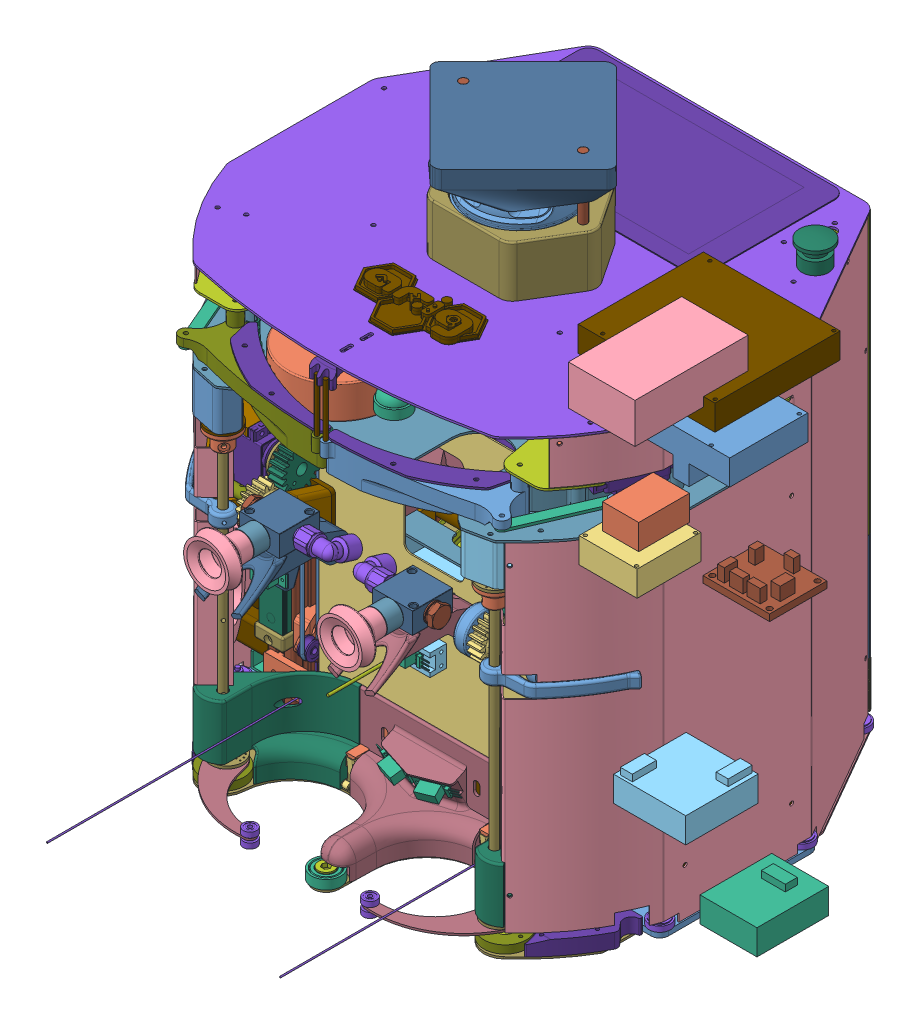
SolidWorks assembly 2019_Gros_robot, configuration Défaut. Lengths in mm. (continued)
Components (placement in the parent): (continued)
- 20181005-1508-1: 20181005-1508 [Défaut] at (-50 277.5 -86.6025) x (0 0 1) z (-1 0 0) size (212.1 303.52 220.42)
  - 20181005-1449-1: 20181005-1449 [Défaut] at (-40 0 0) size (80 80 0) (hidden)
  - 20181005-1520-1: 20181005-1520 [Défaut] at (40 -35 0) x (-0.992278 0.124035 0) z (0 0 -1) size (48.31 18.76 50.57)
  - 20181005-1525-1: 20181005-1525 [Défaut] at (30 -50 0) x (-0.986394 0.164399 0) z (0 0 -1) size (38.41 16.66 50.83)
  - 20181005-1532-1: 20181005-1532 [Défaut] at origin size (84 50 84)
  - Rotule Rose-1: Rotule Rose [aligné] at (33.0169 -69.1373 7) x (0.894203 -0.447662 0) z (-0.447662 -0.894203 0) size (18 6.89 7.5)
    - Rotule Rose piece01-1: Rotule Rose piece01 [Défaut] at origin size (5.4 6 5.4)
    - Rotule Rose piece02-1: Rotule Rose piece02 [Défaut] x (-1 0 0) z (0 0 -1) size (18 5.77 7.5)
  - Rotule noire-2: Rotule noire [Aligné] at (3.5082 -54.3644 7) x (0.894203 -0.447662 0) z (-0.447662 -0.894203 0) size (19 15.5 6.5)
    - Rotule noire piece01-1: Rotule noire piece01 [Défaut] at origin size (6.35 14.5 5.5)
    - Rotule noire piece02-1: Rotule noire piece02 [Défaut] at origin size (19 6 6.5)
  - Rondelle-M3-1: Rondelle-M3 [Défaut] at (40 -35 25) x (0.373687 0.927555 0) z (0 0 1) size (8 8 0.8)
  - EcrouFrein_H-M3-1: EcrouFrein_H-M3 [Défaut] at (40 -35 25.8) x (0.960386 -0.278675 0) z (0 0 1) size (6.35 5.5 4)
  - Rondelle-M3-3: Rondelle-M3 [Défaut] at (30 -50 20.2) x (0.958956 -0.283556 0) z (0 0 1) size (8 8 0.8)
  - Rondelle-M3-4: Rondelle-M3 [Défaut] at (30 -50 25) size (8 8 0.8)
  - EcrouFrein_H-M3-2: EcrouFrein_H-M3 [Défaut] at (30 -50 25.8) x (0.755806 -0.654795 0) z (0 0 1) size (6.35 5.5 4)
  - Rondelle-M3-5: Rondelle-M3 [Défaut] at (40 -35 20.2) x (0.958956 -0.283556 0) z (0 0 1) size (8 8 0.8)
  - Rondelle-M3-6: Rondelle-M3 [Défaut] at (0 -45 22.5) size (8 8 0.8)
  - Rondelle-M3-7: Rondelle-M3 [Défaut] at (0 -45 17.7) x (0.958956 -0.283556 0) z (0 0 1) size (8 8 0.8)
  - Rondelle-M3-8: Rondelle-M3 [Défaut] at (0 -30 22.5) size (8 8 0.8)
  - Rondelle-M3-9: Rondelle-M3 [Défaut] at (0 -30 17.7) x (0.958956 -0.283556 0) z (0 0 1) size (8 8 0.8)
  - EcrouFrein_H-M3-3: EcrouFrein_H-M3 [Défaut] at (0 -45 23.3) x (0.755806 -0.654795 0) z (0 0 1) size (6.35 5.5 4)
  - EcrouFrein_H-M3-4: EcrouFrein_H-M3 [Défaut] at (0 -30 23.3) x (0.755806 -0.654795 0) z (0 0 1) size (6.35 5.5 4)
  - EcrouFrein_H-M3-5: EcrouFrein_H-M3 [Défaut] at (0 -45 -23.3) x (-0.328469 -0.944515 0) z (0 0 -1) size (6.35 5.5 4)
  - Rondelle-M3-10: Rondelle-M3 [Défaut] at (0 -45 -23.3) size (8 8 0.8)
  - Rondelle-M3-11: Rondelle-M3 [Défaut] at (0 -45 -18.5) size (8 8 0.8)
  - Rondelle-M3-12: Rondelle-M3 [Défaut] at (0 -30 -18.5) size (8 8 0.8)
  - Rondelle-M3-13: Rondelle-M3 [Défaut] at (0 -30 -23.3) size (8 8 0.8)
  - EcrouFrein_H-M3-6: EcrouFrein_H-M3 [Défaut] at (0 -30 -23.3) x (-0.328469 -0.944515 0) z (0 0 -1) size (6.35 5.5 4)
  - Rondelle-M3-14: Rondelle-M3 [Défaut] at (40 -35 -25.8) size (8 8 0.8)
  - EcrouFrein_H-M3-7: EcrouFrein_H-M3 [Défaut] at (40 -35 -25.8) x (-0.328469 -0.944515 0) z (0 0 -1) size (6.35 5.5 4)
  - Rondelle-M3-15: Rondelle-M3 [Défaut] at (40 -35 -21) size (8 8 0.8)
  - Rondelle-M3-16: Rondelle-M3 [Défaut] at (30 -50 -21) size (8 8 0.8)
  - Rondelle-M3-17: Rondelle-M3 [Défaut] at (30 -50 -25.8) size (8 8 0.8)
  - EcrouFrein_H-M3-8: EcrouFrein_H-M3 [Défaut] at (30 -50 -25.8) x (-0.328469 -0.944515 0) z (0 0 -1) size (6.35 5.5 4)
  - Palet-1: Palet [Redium] at (0 12.7 0) size (76.2 25.4 76.2)
  - 20181005-2259-1: 20181005-2259 [Défaut] at (-69.4 -270.5 0) size (84 270.5 220.42) (hidden)
  - Palet-2: Palet [Redium] at (-54.2246 -232.142 0) x (0.022904 0.999738 0) z (0 0 1) size (76.2 25.4 76.2)
  - Palet-3: Palet [Redium] at (-52.4793 -155.962 0) x (-0.022904 -0.999738 0) z (0 0 -1) size (76.2 25.4 76.2)
  - Palet-4: Palet [Redium] at (-57 -79.3665 0) x (0.005796 0.999983 0) z (0 0 1) size (76.2 25.4 76.2)
  - 20181006-0057-1: 20181006-0057 [Défaut] at (40 -35 0) size (109.6 110.42 46)
  - 20181006-0127-1: 20181006-0127 [Défaut] at (5.6 -53.5947 -48) size (47 24.09 104)
  - Igus_TK_04_09_Rail_L50-1: Igus_TK_04_09_Rail_L50 [Défaut] at (-10.4 -270.5 0) x (0 0 -1) z (0 1 0) size (9.6 50 6.3)
  - Igus_TK_04_09_coulisseau-1: Igus_TK_04_09_coulisseau [Défaut] at (-78.9 -270.5 0) x (0 0 -1) z (0 1 0) size (20 29 8.3)
  - 20181006-1513-1: 20181006-1513 [Défaut] at (-20.9 -260.5 0) x (0 0 1) z (-1 0 0) size (55 3 30) (hidden)
  - 20181006-1518-1: 20181006-1518 [Défaut] at (-5.9 -265.85 -24) x (0 0 1) z (-1 0 0) size (7.5 7.5 65) (hidden)
  - 20181006-1518-2: 20181006-1518 [Défaut] at (-5.9 -265.85 24) x (0 0 -1) z (-1 0 0) size (7.5 7.5 65) (hidden)
  - Servo_HS-485-HB-1: Servo_HS-485-HB [Default] at (55 -70 -42.29) x (-1 0 0) z (0 0 1) size (19.81 54.15 42.74)
  - Access_HS-485_BrasReglablePartieA-1: Access_HS-485_BrasReglablePartieA [Défaut] at (55 -70 0.45) x (0.039215 0.999231 0) z (0.999231 -0.039215 0) size (10 6 10)
  - Access_HS-485_BrasReglablePartieB-1: Access_HS-485_BrasReglablePartieB [Défaut] at (55.9992 -70.0392 1.45) x (0.039215 0.999231 0) z (0.999231 -0.039215 0) size (7.5 2 30.5)
  - Servo_HS-485-HB-2: Servo_HS-485-HB [Default] at (-17.4 -237.5 -49.74) x (-1 0 0) z (0 0 1) size (19.81 54.15 42.74)
  - microswitchGaletAss-1: microswitchGaletAss [Défaut] at (50 -23 -29.5) x (0 1 0) z (0 0 1) size (21.06 21.1 7)
    - microswitchGalet02-1: microswitchGalet02 [Défaut] at origin size (20 15 7)
    - microswitchGalet01-1: microswitchGalet01 [Défaut] at (1.7099 12.1145 0) x (0.996636 -0.081957 0) z (0 0 1) size (19 9 6)
  - Access_HS-645_BrasRondPetitModele-1: Access_HS-645_BrasRondPetitModele [Défaut] at (-17.4 -237.5 -10) x (0.340211 -0.940349 0) z (-0.940349 -0.340211 0) size (24 5 24)
  - Servo_HS-485-HB-3: Servo_HS-485-HB [Default] at (-17.4 -237.5 -50.26) x (1 0 0) z (0 0 -1) size (19.81 54.15 42.74)
  - Access_HS-645_BrasRondPetitModele-2: Access_HS-645_BrasRondPetitModele [Défaut] at (-17.4 -237.5 -90) x (0.232733 0.972541 0) z (-0.972541 0.232733 0) size (24 5 24)
  - 20190325-2254-1: 20190325-2254 [Défaut] at (-5.9 -256.5 0) x (0 0 1) z (-1 0 0) size (56 23 30)
  - 20190325-2336-1: 20190325-2336 [Défaut] at (-17.4 -237.5 -5.5) x (-0.001924 -0.999998 0) z (0 0 1) size (24 31 4)
  - 20190325-2347-1: 20190325-2347 [Défaut] at (-32.4 -237.4711 -1.5) x (0.865384 -0.50111 0) z (0 0 1) size (33.5 7.5 1.5)
  - 20190326-0009-1: 20190326-0009 [Défaut] at (-5.9 -265.5 25) x (0 0 1) z (-1 0 0) size (8 8 65)
  - 20190326-0009-2: 20190326-0009 [Défaut] at (-5.9 -265.5 -25) x (0 0 1) z (-1 0 0) size (8 8 65)
  - 20190327-2029-1: 20190327-2029 [Défaut] at (-69.4011 -269.4991 -50) size (23.86 187.02 200)
  - 20190327-2138-1: 20190327-2138 [Défaut] at (-17.4 -227.5 -50) size (40 70 54)
  - microswitchGaletAss-2: microswitchGaletAss [Défaut] at (-59.4 -233 47.5) x (0 -1 0) z (0 0 -1) size (21.06 21.1 7)
    - microswitchGalet02-1: microswitchGalet02 [Défaut] at origin size (20 15 7)
    - microswitchGalet01-1: microswitchGalet01 [Défaut] at (1.7099 12.1145 0) x (0.996636 -0.081957 0) z (0 0 1) size (19 9 6)
  - 20190328-2330-1: 20190328-2330 [Défaut] at (-69.4 -270.5 0) size (84 269 20.21)
  - 20190328-2332-1: 20190328-2332 [Défaut] at (-69.4 -270.5 0) size (84 270.5 20)
  - Symétrie20190328-2330-2: Symétrie20190328-2330 [Défaut] at (-69.4 -270.5 -100) size (84 269 20.21)
  - Symétrie20181006-0057-2: Symétrie20181006-0057 [Défaut] at (40 -35 -100) size (109.6 110.42 46)
  - 20181005-1532-2: 20181005-1532 [Défaut] at (0 0 -100) size (84 50 84)
  - Servo_HS-485-HB-4: Servo_HS-485-HB [Default] at (55 -49.85 -57.71) x (-1 0 0) z (0 0 -1) size (19.81 54.15 42.74)
  - Access_HS-485_BrasReglablePartieA-2: Access_HS-485_BrasReglablePartieA [Défaut] at (55 -70 -100.45) x (0.039215 0.999231 0) z (-0.999231 0.039215 0) size (10 6 10)
  - Access_HS-485_BrasReglablePartieB-2: Access_HS-485_BrasReglablePartieB [Défaut] at (55.9992 -70.0392 -101.45) x (-0.039215 -0.999231 0) z (0.999231 -0.039215 0) size (7.5 2 30.5)
  - Rotule Rose-2: Rotule Rose [aligné] at (33.0169 -69.1373 -107) x (0.894203 -0.447662 0) z (0.447662 0.894203 0) size (18 6.89 7.5)
    - Rotule Rose piece01-1: Rotule Rose piece01 [Défaut] at origin size (5.4 6 5.4)
    - Rotule Rose piece02-1: Rotule Rose piece02 [Défaut] x (-1 0 0) z (0 0 -1) size (18 5.77 7.5)
  - Rotule noire-3: Rotule noire [Aligné] at (3.5082 -54.3644 -107) x (0.894203 -0.447662 0) z (0.447662 0.894203 0) size (19 15.5 6.5)
    - Rotule noire piece01-1: Rotule noire piece01 [Défaut] at origin size (6.35 14.5 5.5)
    - Rotule noire piece02-1: Rotule noire piece02 [Défaut] at origin size (19 6 6.5)
  - Symétrie20181006-0127-2: Symétrie20181006-0127 [Défaut] at (5.6 -53.5947 -52) size (47 24.09 104)
  - Igus_TK_04_09_Rail_L50-2: Igus_TK_04_09_Rail_L50 [Défaut] at (-10.4 -270.5 -100) x (0 0 -1) z (0 1 0) size (9.6 50 6.3)
  - Igus_TK_04_09_coulisseau-2: Igus_TK_04_09_coulisseau [Défaut] at (-78.9 -258.8 -100) x (0 0 1) z (0 -1 0) size (20 29 8.3)
  - Symétrie20190325-2254-2: Symétrie20190325-2254 [Défaut] at (-5.9 -256.5 -100) x (0 0 -1) z (1 0 0) size (56 23 30)
  - 20190326-0009-3: 20190326-0009 [Défaut] at (-5.9 -265.5 -125) x (0 0 1) z (-1 0 0) size (8 8 65)
  - 20190326-0009-4: 20190326-0009 [Défaut] at (-5.9 -265.5 -75) x (0 0 1) z (-1 0 0) size (8 8 65)
  - 20190325-2347-2: 20190325-2347 [Défaut] at (-32.4 -237.4711 -100) x (0.865384 -0.50111 0) z (0 0 1) size (33.5 7.5 1.5)
  - 20190325-2336-2: 20190325-2336 [Défaut] at (-17.4 -237.5 -94.5) x (0.001924 0.999998 0) z (0 0 -1) size (24 31 4)
  - EcrouFrein_H-M3-9: EcrouFrein_H-M3 [Défaut] at (40 -35 -74.2) x (0.328469 0.944515 0) z (0 0 1) size (6.35 5.5 4)
  - EcrouFrein_H-M3-10: EcrouFrein_H-M3 [Défaut] at (0 -30 -76.7) x (0.328469 0.944515 0) z (0 0 1) size (6.35 5.5 4)
  - Rondelle-M3-18: Rondelle-M3 [Défaut] at (0 -30 -77.5) size (8 8 0.8)
  - Rondelle-M3-19: Rondelle-M3 [Défaut] at (0 -45 -77.5) size (8 8 0.8)
  - EcrouFrein_H-M3-11: EcrouFrein_H-M3 [Défaut] at (0 -45 -76.7) x (0.328469 0.944515 0) z (0 0 1) size (6.35 5.5 4)
  - Rondelle-M3-20: Rondelle-M3 [Défaut] at (30 -50 -75) size (8 8 0.8)
  - EcrouFrein_H-M3-12: EcrouFrein_H-M3 [Défaut] at (30 -50 -74.2) x (0.328469 0.944515 0) z (0 0 1) size (6.35 5.5 4)
  - Rondelle-M3-21: Rondelle-M3 [Défaut] at (30 -50 -79.8) size (8 8 0.8)
  - 20181005-1525-2: 20181005-1525 [Défaut] at (30 -50 -100) x (-0.986394 0.164399 0) z (0 0 -1) size (38.41 16.66 50.83)
  - Rondelle-M3-22: Rondelle-M3 [Défaut] at (40 -35 -75) size (8 8 0.8)
  - Rondelle-M3-23: Rondelle-M3 [Défaut] at (40 -35 -79.8) size (8 8 0.8)
  - 20181005-1520-2: 20181005-1520 [Défaut] at (40 -35 -100) x (-0.992278 0.124035 0) z (0 0 -1) size (48.31 18.76 50.57)
  - Rondelle-M3-24: Rondelle-M3 [Défaut] at (0 -30 -82.3) size (8 8 0.8)
  - Rondelle-M3-25: Rondelle-M3 [Défaut] at (0 -45 -82.3) size (8 8 0.8)
  - Rondelle-M3-26: Rondelle-M3 [Défaut] at (0 -45 -118.5) x (0.958956 -0.283556 0) z (0 0 1) size (8 8 0.8)
  - Rondelle-M3-27: Rondelle-M3 [Défaut] at (0 -45 -123.3) size (8 8 0.8)
  - EcrouFrein_H-M3-13: EcrouFrein_H-M3 [Défaut] at (0 -45 -123.3) x (-0.755806 0.654795 0) z (0 0 -1) size (6.35 5.5 4)
  - Rondelle-M3-28: Rondelle-M3 [Défaut] at (0 -30 -123.3) size (8 8 0.8)
  - EcrouFrein_H-M3-14: EcrouFrein_H-M3 [Défaut] at (0 -30 -123.3) x (-0.755806 0.654795 0) z (0 0 -1) size (6.35 5.5 4)
  - Rondelle-M3-29: Rondelle-M3 [Défaut] at (30 -50 -121) x (0.958956 -0.283556 0) z (0 0 1) size (8 8 0.8)
  - Rondelle-M3-30: Rondelle-M3 [Défaut] at (30 -50 -125.8) size (8 8 0.8)
  - EcrouFrein_H-M3-15: EcrouFrein_H-M3 [Défaut] at (30 -50 -125.8) x (-0.755806 0.654795 0) z (0 0 -1) size (6.35 5.5 4)
  - Rondelle-M3-31: Rondelle-M3 [Défaut] at (40 -35 -121) x (0.958956 -0.283556 0) z (0 0 1) size (8 8 0.8)
  - Rondelle-M3-32: Rondelle-M3 [Défaut] at (40 -35 -125.8) x (0.373687 0.927555 0) z (0 0 1) size (8 8 0.8)
  - EcrouFrein_H-M3-16: EcrouFrein_H-M3 [Défaut] at (40 -35 -125.8) x (-0.960386 0.278675 0) z (0 0 -1) size (6.35 5.5 4)
  - Rondelle-M3-33: Rondelle-M3 [Défaut] at (0 -30 -118.5) x (0.958956 -0.283556 0) z (0 0 1) size (8 8 0.8)
  - microswitchGaletAss-3: microswitchGaletAss [Défaut] at (50 -23 -70.5) x (0 1 0) z (0 0 1) size (21.06 21.1 7)
    - microswitchGalet02-1: microswitchGalet02 [Défaut] at origin size (20 15 7)
    - microswitchGalet01-1: microswitchGalet01 [Défaut] at (1.7099 12.1145 0) x (0.996636 -0.081957 0) z (0 0 1) size (19 9 6)
  - microswitchGaletAss-4: microswitchGaletAss [Défaut] at (-59.4 -233 -147.5) x (0 -1 0) z (0 0 -1) size (21.06 21.1 7)
    - microswitchGalet02-1: microswitchGalet02 [Défaut] at origin size (20 15 7)
    - microswitchGalet01-1: microswitchGalet01 [Défaut] at (1.7099 12.1145 0) x (0.996636 -0.081957 0) z (0 0 1) size (19 9 6)
- 20181006-0254-1: 20181006-0254 [Défaut] at (0 343.5 -160.0025) size (213 210 4)
- Palet-1: Palet [Redium] at (-50 12.7 119.5978) size (76.2 25.4 76.2) (hidden)
- Raspberry pi3 Screen assembly-1: Raspberry pi3 Screen assembly [Défaut] at (-26.2349 344.907 -108.8519) x (0.999654 0 -0.026321) z (0 1 0) size (195.4 115.39 39.45)
- Carte alimentation convertisseur-1: Carte alimentation convertisseur [Défaut] at (195.1731 449.8125 151.3603) size (102.6 19 94) (hidden)
- Interf Raspi-1: Interf Raspi [Défaut] at (205.7046 396.6201 128.2669) size (80.1 34 58.6) (hidden)
- Capteurs Analogique-1: Capteurs Analogique [Défaut] at (234.5762 364.7789 172.5689) size (27.2 19 38.1) (hidden)
- Capteurs Numerique-1: Capteurs Numerique [Défaut] at (209.8881 326.819 165.4886) size (43.6 19 47.8) (hidden)
- SD21-1: SD21 [Défaut] at (239.2416 462.0315 160.3108) size (50 30 85) (hidden)
- Carte codeur v2-1: Carte codeur v2 [Défaut] at (181.4763 130.2292 111.0518) size (54.1 39 54.4) (hidden)
- Carte codeur v1-1: Carte codeur v1 [Défaut] at (219.0947 57.0207 83.9025) size (42.8 24 53.9) (hidden)
- pompe air 12v SFE-2: pompe air 12v SFE [Défaut] at (20.3606 32 -38) size (38 60 92)
- BillePorteuse2019-1: BillePorteuse2019 [Défaut] at (105.917 0 116.9526) x (0.630519 0 -0.776174) z (0.776174 0 0.630519) size (16 10 16)
- microswitchGaletAss-1: microswitchGaletAss [Défaut] at (50 29 66) x (0 -1 0) z (-1 0 0) size (21.06 21.1 7)
  - microswitchGalet02-1: microswitchGalet02 [Défaut] at origin size (20 15 7)
  - microswitchGalet01-1: microswitchGalet01 [Défaut] at (1.7099 12.1145 0) x (0.996636 -0.081957 0) z (0 0 1) size (19 9 6)
- Roulement_d3xd10xe4-1: Roulement_d3xd10xe4 [Défaut] at (45.0929 15.95 157.5553) x (0 1 0) z (-0.541709 0 -0.840566) size (4 10 10)
- roulement-1: roulement [Défaut] at (0 11.5 145.4518) x (0 -1 0) z (0.861176 0 0.508306) size (7 22 22)
- Servo_HS-485-HB-1: Servo_HS-485-HB [Default] at (148.2228 335.79 52.8032) x (-0.95652 0 -0.291667) z (0 -1 0) size (19.81 54.15 42.74)
- Access_HS-485_BrasReglablePartieB-1: Access_HS-485_BrasReglablePartieB [Défaut] at (148.4345 292.05 51.8259) x (0.977331 0 0.211718) z (0.211718 0 -0.977331) size (7.5 2 30.5)
- Access_HS-485_BrasReglablePartieA-1: Access_HS-485_BrasReglablePartieA [Défaut] at (148.2228 293.05 52.8032) x (0.977331 0 0.211718) z (0.211718 0 -0.977331) size (10 6 10)
- 20190123-2208-1: 20190123-2208 [Défaut] at (0 8.1 145.4518) size (11.85 7.9 11.85)
- Electrovanne12VDC-1: Electrovanne12VDC [Défaut] at (47 164.0788 27.5) x (0 -1 0) z (0 0 1) size (36.5 64 22)
- CapteurVide_CKD_PPE-V01A-H6-B-1: CapteurVide_CKD_PPE-V01A-H6-B [Défaut] at (90 114.0788 27.5) x (0 -1 0) z (0 0 1) size (37 43 15)
- CarteVentillo-1: CarteVentillo [Défaut] at (248.165 281.582 64.2045) size (50 15 43) (hidden)
- 20190208-2148-1: 20190208-2148 [Défaut] at (102 60.4 120.9526) x (0.640285 0 0.768138) z (0 1 0) size (6 6 175)
- 20190208-2207-1: 20190208-2207 [Défaut] at (102.5 18.75 117.5) x (-0.820101 0 0.572218) z (-0.572218 0 -0.820101) size (86 1.5 31.58)
- Roulement_d3xd10xe4-2: Roulement_d3xd10xe4 [Défaut] at (45.0929 23.05 157.5553) x (0 1 0) z (-0.268999 0 0.963141) size (4 10 10)
- Servo_HS-85-BB-1: Servo_HS-85-BB [Défaut] at (102.5 25.85 117.5) x (1 0 0) z (0 -1 0) size (13 41.3 34.1)
- 20190212-2200-1: 20190212-2200 [Défaut] at (-50 7 120) size (239.52 60.05 68.05)
- 20190214-0012-1: 20190214-0012 [Défaut] at (105.917 8.7 116.9526) x (0.866025 0 -0.5) z (0.5 0 0.866025) size (32 10 32)
- Access_HS-645_BrasRondPetitModele-1: Access_HS-645_BrasRondPetitModele [Défaut] at (102.5 24.75 117.5) x (-0.643539 0 0.765413) z (0.765413 0 0.643539) size (24 5 24)
- 20190208-2207-2: 20190208-2207 [Défaut] at (102.5 18.75 117.5) x (0.794361 0 -0.607446) z (0.607446 0 0.794361) size (86 1.5 31.58) (hidden)
- 20170416-2304-1: 20170416-2304 [Défaut] at (12.2889 46.5676 67.2799) x (0.965926 0.109382 -0.23457) z (0.258819 -0.408218 0.875426) size (30.6 16 70.4)
  - SupportCapteurPololu-1: SupportCapteurPololu [Défaut] at origin size (30 16 12.5) (hidden)
  - pololu gp2y0d805-1: pololu gp2y0d805 [Défaut] at (-14.5 -4.5 10.8) size (30.1 9 11.8)
  - faisceau pololu gp2y0d-1: faisceau pololu gp2y0d [5cm] at (-3.9 0 20.4) size (2 2 50) (hidden)
- 20190219-0006-1: 20190219-0006 [Défaut] at (0 7 0) size (30.83 11 59.43)
- Roulement_d3xd10xe4-3: Roulement_d3xd10xe4 [Défaut] at (158.1053 15.95 74.9788) x (0 1 0) z (-0.541709 0 -0.840566) size (4 10 10) (hidden)
- 20190219-0101-1: 20190219-0101 [Défaut] at (130 51.0678 50) x (0 0 -1) z (1 0 0) size (22 20 34.5)
- 20190219-0101-2: 20190219-0101 [Défaut] at (130 51.0678 -50) x (0 0 1) z (1 0 0) size (22 20 34.5)
- 20190220-2148-1: 20190220-2148 [Défaut] at (102 181.4 120.9526) x (0.406737 0 -0.913545) z (0.913545 0 0.406737) size (78.13 10.25 45.74)
- Servo_HS-85-BB-2: Servo_HS-85-BB [Défaut] at (102 246 120.9526) x (0.5 0 0.866025) z (0 -1 0) size (13 41.3 34.1)
- Access_HS-645_BrasRondPetitModele-2: Access_HS-645_BrasRondPetitModele [Défaut] at (102 244.9 120.9526) x (-0.940804 0 0.338952) z (0.338952 0 0.940804) size (24 5 24)
- 20190221-0033-1: 20190221-0033 [Défaut] at (102 240.4 120.9526) x (-0.640285 0 -0.768138) z (-0.768138 0 0.640285) size (24 15 24)
- 20190221-0152-1: 20190221-0152 [Défaut] at (0 312.2 0) x (-1 0 0) z (0 0 1) size (65.17 50 53.91)
- Carter2019-1: Carter2019 [Défaut] at (0 7 0) size (63.71 336 283.98)
- 20190223-1730-1: 20190223-1730 [Défaut] at (-0.1299 256 0.1276) size (48.99 30 36.97)
- 20170416-2304-2: 20170416-2304 [Défaut] at (-12.2889 46.5676 67.2799) x (-0.965926 0.109382 -0.23457) z (-0.258819 -0.408218 0.875426) size (30.6 16 70.4)
  - SupportCapteurPololu-1: SupportCapteurPololu [Défaut] at origin size (30 16 12.5) (hidden)
  - pololu gp2y0d805-1: pololu gp2y0d805 [Défaut] at (-14.5 -4.5 10.8) size (30.1 9 11.8)
  - faisceau pololu gp2y0d-1: faisceau pololu gp2y0d [5cm] at (-3.9 0 20.4) size (2 2 50) (hidden)
- 20190225-2214-1: 20190225-2214 [Défaut] at (118.6064 288.5 132.1497) x (0.396167 0 -0.918178) z (0.918178 0 0.396167) size (71 2 8)
- Robot2019_plaque elec-1: Robot2019_plaque elec [Défaut] at (0 309.5 0) size (330 1.5 265.02)
- Robot2019_plaque superieure-2: Robot2019_plaque superieure [Défaut] at (0 343.5 0) size (330 1.5 305)
- 20161105-0900-1: 20161105-0900 [Défaut] at (0 345 0) size (105 35.5 75)
- 20190313-2117-1: 20190313-2117 [Défaut] at (0 430 -2.5) x (-1 0 0) z (0 0 1) size (135.87 27.01 134.45)
- 20161106-1538-1: 20161106-1538 [Défaut] at (-45 350 -2.5) size (6 80 6)
- 20161106-1538-2: 20161106-1538 [Défaut] at (45 350 -2.5) size (6 80 6)
- 20170416-2304-3: 20170416-2304 [Défaut] at (-120 226 -15) x (0 0 -1) z (0 1 0) size (30.6 16 70.4)
  - SupportCapteurPololu-1: SupportCapteurPololu [Défaut] at origin size (30 16 12.5) (hidden)
  - pololu gp2y0d805-1: pololu gp2y0d805 [Défaut] at (-14.5 -4.5 10.8) size (30.1 9 11.8)
  - faisceau pololu gp2y0d-1: faisceau pololu gp2y0d [5cm] at (-3.9 0 20.4) size (2 2 50) (hidden)
- Adafruit_TCS34725-1: Adafruit_TCS34725 [Défaut] at (-106.6 273 31) x (0 0 -1) z (0 1 0) size (20.5 20.4 5)
- 20190227-2336-1: 20190227-2336 [Défaut] at (-120 256.5 40) x (-1 0 0) z (0 0 -1) size (17 25 31.5)
- 20190228-0009-1: 20190228-0009 [Défaut] at (0 165.5788 39.25) x (0 0 -1) z (-1 0 0) size (19.5 19.5 255)
- Robot2015_supportServo02-1: Robot2015_supportServo02 [Défaut] at (-34 217.5 -3.6025) x (0 0 -1) z (1 0 0) size (38 65 1.5)
- 20190301-2106-1: 20190301-2106 [Défaut] at (47.184 337.04 -102.825) x (-1 0 0) z (0 0 -1) size (55 8.5 82)
- 20190301-2139-1: 20190301-2139 [Défaut] at (0 343.5 0) size (18.21 12.25 42)
- LogoARIG2-1: LogoARIG2 [Défaut] at (-42.5 345 104) x (1 0 0) z (0 1 0) size (88.08 45.8 6.03)
- GP2D-2: GP2D [Défaut] at (75 287.5 -145) x (-1 0 0) z (0 0 1) size (44.5 15.5 19)
- 20190301-2106-2: 20190301-2106 [Défaut] at (-63.016 337.04 -102.825) size (55 8.5 82)
- LogoARIG2-2: LogoARIG2 [Défaut] at (42.5 244.5 -160.0025) x (-1 0 0) z (0 0 -1) size (88.08 45.8 6.03)
- 20190308-1510-1: 20190308-1510 [Défaut] at (0 336.5 0) size (33.55 41 203.81)
- interrupteur principal-1: interrupteur principal [Défaut] at (145.1715 323 -71.7856) x (0.5 0 0.866025) z (0 1 0) size (32 33.35 25)
- 20190308-2149-1: 20190308-2149 [Défaut] at (0 343.5 0) x (-1 0 0) z (0 0 1) size (43.23 7 234.12)
- 20190309-0049-1: 20190309-0049 [Défaut] at (0 311 43) size (178.08 32 17)
- 20190309-0127_Corniere_15.5x27.5x1.5-1: 20190309-0127_Corniere_15.5x27.5x1.5 [Défaut] at (-130 276 -59) x (-1 0 0) z (0 0 1) size (27.5 15.5 118)
- Ventilo-2: Ventilo [Défaut] at (75 318.5 -156.0025) size (40 40 11.91)
- TelemetreTOF_RB-Mce-01-1: TelemetreTOF_RB-Mce-01 [Défaut] at (-74.5065 272.4886 -143) x (0 0 1) z (0.139173 -0.990268 0) size (25 30.5 210)
- Ventilo-3: Ventilo [Défaut] at (0 318.5 -156.0025) size (40 40 11.91)
- Ventilo-4: Ventilo [Défaut] at (-75 318.5 -156.0025) size (40 40 11.91)
- 20190314-1109-1: 20190314-1109 [Défaut] at (-74.5065 272.4886 -143) x (0 0 1) z (-0.990268 -0.139173 0) size (25 4.81 20)
- 20181006-0255-1: 20181006-0255 [Défaut] at (0 133.2 -160.0025) size (213 80 4)
- Palet-2: Palet [Redium] at (51.9 38.1 -143.8025) x (0 1 0) z (-1 0 0) size (76.2 25.4 76.2) (hidden)
- TelemetreTOF_RB-Mce-01-2: TelemetreTOF_RB-Mce-01 [Défaut] at (87.5 42 64.5) size (25 30.5 210)
- 20190331-1440-1: 20190331-1440 [Défaut] at (87.5 42 64.5) x (1 0 0) z (0 1 0) size (55.5 6 20)
- 20190331-1545-1: 20190331-1545 [Défaut] at (0 383.5 -2.5) x (-1 0 0) z (0 0 1) size (110 38.3 83)
- 20190331-1640-1: 20190331-1640 [Défaut] at (0 257 22.5) size (90 54 43)
- 20190309-0128-1: 20190309-0128 [Défaut] at (-130 276 -59) x (-1 0 0) z (0 0 1) size (27.02 16 119.7)
- SupportCapteurPololuSpecial2019-1: SupportCapteurPololuSpecial2019 [Défaut] at (-120 226 -15) x (0 0 -1) z (0 1 0) size (41.3 16 24)
- Robot2015_BaseRoulante_piece15-1: Robot2015_BaseRoulante_piece15 [Défaut] at (-95 79.5 -60) x (0 0 -1) z (1 0 0) size (40 40 190)
- Symétrie20190219-0006-2: Symétrie20190219-0006 [Défaut] at (0 7 0) x (-1 0 0) z (0 0 -1) size (30.83 11 59.43)
- microswitchGaletAss-2: microswitchGaletAss [Défaut] at (-50 29 66) x (0 -1 0) z (-1 0 0) size (21.06 21.1 7)
  - microswitchGalet02-1: microswitchGalet02 [Défaut] at origin size (20 15 7)
  - microswitchGalet01-1: microswitchGalet01 [Défaut] at (1.7099 12.1145 0) x (0.996636 -0.081957 0) z (0 0 1) size (19 9 6)
- 20190208-2207-3: 20190208-2207 [Défaut] at (-102.5 20.25 117.5) x (0.820101 0 0.572218) z (0.572218 0 -0.820101) size (86 1.5 31.58)
- Roulement_d3xd10xe4-4: Roulement_d3xd10xe4 [Défaut] at (-45.0929 23.05 157.5553) x (0 1 0) z (-0.268999 0 -0.963141) size (4 10 10)
- Roulement_d3xd10xe4-5: Roulement_d3xd10xe4 [Défaut] at (-45.0929 15.95 157.5553) x (0 1 0) z (-0.541709 0 0.840566) size (4 10 10)
- Access_HS-645_BrasRondPetitModele-3: Access_HS-645_BrasRondPetitModele [Défaut] at (-102.5 19.75 117.5) x (0.643539 0 0.765413) z (-0.765413 0 0.643539) size (24 5 24)
- 20190214-0012-2: 20190214-0012 [Défaut] at (-105.917 8.7 116.9526) x (0.866025 0 0.5) z (-0.5 0 0.866025) size (32 10 32)
- BillePorteuse2019-2: BillePorteuse2019 [Défaut] at (-105.917 0 116.9526) x (-0.630519 0 -0.776174) z (0.776174 0 -0.630519) size (16 10 16)
- 20190208-2148-2: 20190208-2148 [Défaut] at (-102 235.4 120.9526) x (-0.640285 0 0.768138) z (0 -1 0) size (6 6 175)
- 20190220-2148-2: 20190220-2148 [Défaut] at (-102 181.4 120.9526) x (-0.406737 0 -0.913545) z (-0.913545 0 0.406737) size (78.13 10.25 45.74)
- 20190221-0033-2: 20190221-0033 [Défaut] at (-102 240.4 120.9526) x (-0.640285 0 0.768138) z (0.768138 0 0.640285) size (24 15 24)
- SymétrieAccess_HS-645_BrasRondPetitModele-4: SymétrieAccess_HS-645_BrasRondPetitModele [Défaut] at (-102 244.9 120.9526) x (0.940804 0 0.338952) z (0.338952 0 -0.940804) size (24 5 24)
- Symétrie20190223-1730-2: Symétrie20190223-1730 [Défaut] at (0.1299 256 0.1276) x (-1 0 0) z (0 0 -1) size (48.99 30 36.97)
- Servo_HS-85-BB-3: Servo_HS-85-BB [Défaut] at (-102.5 25.85 101.5) x (-1 0 0) z (0 -1 0) size (13 41.3 34.1)
- Symétrie20190331-1440-2: Symétrie20190331-1440 [Défaut] at (-87.5 42 64.5) x (-1 0 0) z (0 -1 0) size (55.5 6 20)
- Servo_HS-85-BB-4: Servo_HS-85-BB [Défaut] at (-102 246 120.9526) x (0.5 0 -0.866025) z (0 -1 0) size (13 41.3 34.1)
- Servo_HS-485-HB-2: Servo_HS-485-HB [Default] at (-148.2228 335.79 52.8032) x (-0.95652 0 0.291667) z (0 -1 0) size (19.81 54.15 42.74)
- Access_HS-485_BrasReglablePartieA-2: Access_HS-485_BrasReglablePartieA [Défaut] at (-148.2228 293.05 52.8032) x (-0.977331 0 0.211718) z (0.211718 0 0.977331) size (10 6 10)
- Access_HS-485_BrasReglablePartieB-2: Access_HS-485_BrasReglablePartieB [Défaut] at (-148.4345 292.05 51.8259) x (0.977331 0 -0.211718) z (-0.211718 0 -0.977331) size (7.5 2 30.5)
- 20190225-2214-2: 20190225-2214 [Défaut] at (-118.6064 288.5 132.1497) x (-0.396167 0 -0.918178) z (0.918178 0 -0.396167) size (71 2 8)
- 20190309-0128-2: 20190309-0128 [Défaut] at (130 276 58.6854) x (1 0 0) z (0 0 -1) size (27.02 16 119.7)
- 20190309-0127_Corniere_15.5x27.5x1.5-2: 20190309-0127_Corniere_15.5x27.5x1.5 [Défaut] at (130 276 59) x (1 0 0) z (0 0 -1) size (27.5 15.5 118)
- TelemetreTOF_RB-Mce-01-3: TelemetreTOF_RB-Mce-01 [Défaut] at (-87.5 42 64.5) size (25 30.5 210)
- 20190219-0101-3: 20190219-0101 [Défaut] at (-130 51.0678 -50) x (0 0 1) z (-1 0 0) size (22 20 34.5)
- 20190219-0101-4: 20190219-0101 [Défaut] at (-130 51.0678 50) x (0 0 -1) z (-1 0 0) size (22 20 34.5)
- 2019CarterAvant-1: 2019CarterAvant [Défaut] at (0 56.5 64.5) size (173 218 1)
- SymétrieCarter2019-2: SymétrieCarter2019 [Défaut] at (0 7 0) x (-1 0 0) z (0 0 -1) size (63.71 336 283.98)
- Legris_EQUERRE-OSCILLANTE_3159_06_10-2: Legris_EQUERRE-OSCILLANTE_3159_06_10 [Défaut] at (45 114.0788 27.5) x (0 0.860608 -0.509267) z (0 0.509267 0.860608) size (28 34.3 15.01)
- Legris_NourriceCroix_3312_00_10-2: Legris_NourriceCroix_3312_00_10 [Défaut] at (55 114.0788 35.5) x (1 0 0) z (0 0 -1) size (30 30 16)
- 20190415-2222-1: 20190415-2222 [Défaut] at (0 159.0788 40) size (45 10 22)
- Legris_NourriceCroix_3312_00_10-3: Legris_NourriceCroix_3312_00_10 [Défaut] at (-55 114.0788 19.5) x (-1 0 0) z (0 0 1) size (30 30 16)
- Legris_EQUERRE-OSCILLANTE_3159_06_10-3: Legris_EQUERRE-OSCILLANTE_3159_06_10 [Défaut] at (-45 114.0788 27.5) x (0 0.860608 -0.509267) z (0 -0.509267 -0.860608) size (28 34.3 15.01)
- CapteurVide_CKD_PPE-V01A-H6-B-2: CapteurVide_CKD_PPE-V01A-H6-B [Défaut] at (-90 114.0788 27.5) x (0 -1 0) z (0 0 -1) size (37 43 15)
- Electrovanne12VDC-2: Electrovanne12VDC [Défaut] at (-47 164.0788 27.5) x (0 -1 0) z (0 0 -1) size (36.5 64 22)
- 20190415-2329-1: 20190415-2329 [Défaut] at (-70.5 128.5788 38.5) x (1 0 0) z (0 1 0) size (140 5 30)
Mates (geometry in assembly coordinates):
- Coïncidente1: coincident aligned: line of Robot2019_profiléX20_02-1 through (-110 276 58) axis (0 0 -1); line of Robot2019_profiléX20_02-2 through (-110 276 -53.3) axis (0 0 -1)
- Coïncidente2: coincident aligned: line of Robot2019_profiléX20_02-3 through (110 276 53.3) axis (0 0 1); line of Robot2019_profiléX20_02-4 through (110 276 -58) axis (0 0 1)
- Coïncidente3: coincident aligned: line of Robot2019_profiléX20_02-1 through (-123.3 276 40) axis (-1 0 0); line of Robot2019_profiléX20_02-3 through (128 276 40) axis (-1 0 0)
- Coïncidente4: coincident aligned: line of Robot2019_profiléX20_02-2 through (-128 276 -40) axis (1 0 0); line of Robot2019_profiléX20_02-4 through (123.3 276 -40) axis (1 0 0)
- Coïncidente5: coincident anti-aligned: plane of Robot2017_BaseRoulante-1/Robot2015_BaseRoulante_piece01-1 through (0 11 0) normal (0 1 0); plane of Robot2019_profiléX20_02-1 through (-110.8 11 53.3) normal (0 -1 0)
- Coaxiale1: concentric aligned: cylinder of Robot2017_BaseRoulante-1/Robot2015_BaseRoulante_piece01-1 through (-120 7 50) axis (0 1 0) radius 2.5; cylinder of Robot2019_profiléX20_02-1 through (-120 11 50) axis (0 1 0) radius 2.15
- Coaxiale2: concentric aligned: cylinder of Robot2017_BaseRoulante-1/Robot2015_BaseRoulante_piece01-1 through (120 7 50) axis (0 1 0) radius 2.5; cylinder of Robot2019_profiléX20_02-3 through (120 11 50) axis (0 1 0) radius 2.15
- Coaxiale3: concentric aligned: cylinder of Robot2017_BaseRoulante-1/Robot2015_BaseRoulante_piece01-1 through (-120 7 -50) axis (0 1 0) radius 2.5; cylinder of Robot2019_profiléX20_02-2 through (-120 11 -50) axis (0 1 0) radius 2.15
- Coïncidente6: coincident anti-aligned: plane of Robot2017_BaseRoulante-1/Robot2015_BaseRoulante_piece01-1 through (0 7 0) normal (0 -1 0); plane of Robot2019_plaque bille porteuseAvant-1 through (0 7 0) normal (0 1 0)
- Coaxiale4: concentric anti-aligned: cylinder of Robot2017_BaseRoulante-1/Robot2015_BaseRoulante_piece01-1 through (-70 7 45) axis (0 1 0) radius 1; cylinder of Robot2019_plaque bille porteuseAvant-1 through (-70 7 45) axis (0 -1 0) radius 1.5
- Coaxiale5: concentric anti-aligned: cylinder of Robot2017_BaseRoulante-1/Robot2015_BaseRoulante_piece01-1 through (70 7 45) axis (0 1 0) radius 1; cylinder of Robot2019_plaque bille porteuseAvant-1 through (70 7 45) axis (0 -1 0) radius 1.5
- Coïncidente7: coincident anti-aligned: plane of Robot2017_BaseRoulante-1/Robot2015_BaseRoulante_piece01-1 through (0 7 0) normal (0 -1 0); plane of Robot2019_plaque bille porteuse Arriere-1 through (100.765 7 -153.5) normal (0 1 0)
- Coaxiale6: concentric anti-aligned: cylinder of Robot2017_BaseRoulante-1/Robot2015_BaseRoulante_piece01-1 through (-140 7 -45) axis (0 1 0) radius 1; cylinder of Robot2019_plaque bille porteuse Arriere-1 through (-140 7 -45) axis (0 -1 0) radius 1.5
- Coaxiale7: concentric anti-aligned: cylinder of Robot2017_BaseRoulante-1/Robot2015_BaseRoulante_piece01-1 through (140 7 -45) axis (0 1 0) radius 1; cylinder of Robot2019_plaque bille porteuse Arriere-1 through (140 7 -45) axis (0 -1 0) radius 1.5
- Coïncidente8: coincident anti-aligned: plane of Robot2019_profiléX20_02-1 through (-110.8 276 53.3) normal (0 1 0); plane of Robot2019_plaque du dessus-1 through (0 276 -355) normal (0 -1 0)
- Coïncidente13: coincident aligned: plane of bille porteuse-3; plane of assembly through (0 0 0) normal (0 1 0)
- Coaxiale14: concentric aligned: cylinder of Robot2019_plaque bille porteuse Arriere-1 through (-94.1254 7 -100) axis (0 -1 0) radius 1.5; cylinder of bille porteuse-3/Robot2015_support bille porteuse-1 through (-94.1254 21.5 -100) axis (0 -1 0) radius 1.5
- Coaxiale15: concentric aligned: cylinder of Robot2019_plaque bille porteuse Arriere-1 through (-111.446 7 -130) axis (0 -1 0) radius 1.5; cylinder of bille porteuse-3/Robot2015_support bille porteuse-1 through (-111.446 21.5 -130) axis (0 -1 0) radius 1.5
- Coïncidente33: coincident anti-aligned: plane of Robot2019_plaque bille porteuse Arriere-1 through (100.765 7 -153.5) normal (0 1 0); plane of Robot2015_roulementAngle-2 through (-100.765 7 -153.5) normal (0 -1 0)
- Coïncidente34: coincident anti-aligned: plane of Robot2019_plaque bille porteuse Arriere-1 through (100.765 7 -153.5) normal (0 1 0); plane of Robot2015_roulementAngle-1 through (100.765 7 -153.5) normal (0 -1 0)
- Coaxiale21: concentric aligned: cylinder of Robot2019_plaque bille porteuse Arriere-1 through (100.765 7 -153.5) axis (0 -1 0) radius 1.5; cylinder of Robot2015_roulementAngle-1 through (100.765 11.75 -153.5) axis (0 -1 0) radius 8
- Coaxiale22: concentric aligned: cylinder of Robot2019_plaque bille porteuse Arriere-1 through (-100.765 7 -153.5) axis (0 -1 0) radius 1.5; cylinder of Robot2015_roulementAngle-2 through (-100.765 11.75 -153.5) axis (0 -1 0) radius 8
- Distance54: distance = 170 mm anti-aligned: plane of batterieLIPO-1 through (-65 146 -110) normal (0 0 -1); plane of Robot2019_profiléX20_02-1 through (-116.7 11 60) normal (0 0 1)
- Distance55: distance = 220 mm anti-aligned: plane of Robot2019_profiléX20_02-1 through (-130 11 53.3) normal (-1 0 0); plane of batterieLIPO-1 through (90 146 -76) normal (1 0 0)
- Distance60: distance = 135 mm aligned: plane of batterieLIPO-1 through (-65 146 -76) normal (0 1 0); plane of Robot2017_BaseRoulante-1/Robot2015_BaseRoulante_piece01-1 through (0 11 0) normal (0 1 0)
- Coaxiale23: concentric anti-aligned: cylinder of Robot2019_plaque du dessus-1 through (0 267.5 0) axis (0 1 0) radius 27; cylinder of 20180929-0119-1/20181010-0239-1 through (0 306 0) axis (0 -1 0) radius 49
- Coïncidente98: coincident aligned: plane of Robot2019_plaque du dessus-1 through (0 277.5 -355) normal (0 1 0); plane of 20180929-0119-1
- Parallèle3: parallel anti-aligned: plane of 20180929-0119-1 through (0 277.5 0) normal (0 0 -1); plane of assembly through (0 0 0) normal (0 0 1)
- Coïncidente99: coincident aligned: plane of 20181001-1750-1 through (0 0 0) normal (0 0 1); plane of assembly through (0 0 0) normal (0 0 1)
- Coïncidente100: coincident aligned: plane of 20181001-1750-1 through (0 0 0) normal (0 1 0); plane of assembly through (0 0 0) normal (0 1 0)
- Coïncidente101: coincident aligned: plane of 20181001-1750-1 through (0 0 0) normal (1 0 0); plane of assembly through (0 0 0) normal (1 0 0)
- Coïncidente102: coincident anti-aligned: plane of Robot2019_plaque bille porteuseAvant-1 through (0 7 0) normal (0 1 0); plane of 20181001-2148-1 through (-89.8589 7 116.7694) normal (0 -1 0)
- Parallèle4: parallel anti-aligned: plane of Robot2017_BaseRoulante-1/Robot2015_BaseRoulante_piece01-1 through (0 11 60) normal (0 0 1); plane of 20181001-2148-1 through (-82.6586 29 65) normal (0 0 -1)
- Coaxiale24: concentric: cylinder of Robot2019_plaque bille porteuseAvant-1 through (-50 7 120) axis (0 -1 0) radius 40; point of 20181001-2148-1
- Coïncidente104: coincident aligned: plane of Robot2019_plaque du dessus-1 through (0 277.5 -355) normal (0 1 0); plane of 20181002-0030-1/20181002-0031-1
- Coaxiale26: concentric: cylinder of Robot2019_plaque du dessus-1 through (0 267.5 0) axis (0 1 0) radius 27; point of 20181002-0030-1/20181002-0031-1
- Angle1: planar angle = 0.759218 rad aligned: plane of 20181002-0030-1/20181002-0031-1 through (0 277.5 0) normal (-0.688355 0 0.725374); plane of assembly through (0 0 0) normal (0 0 1)
- Coïncidente105: coincident anti-aligned: plane of Robot2019_plaque du dessus-1 through (0 277.5 -355) normal (0 1 0); plane of 20181002-0216-1/20181002-0217-1 through (0 277.5 0) normal (0 -1 0)
- Symétrique1: symmetric aligned: cylinder of Robot2019_plaque du dessus-1 through (-106.7731 275.999 106.7731) axis (0 1 0) radius 1.5; cylinder of 20181002-0216-1/20181002-0217-1 through (-106.7731 430.1481 106.7731) axis (0 -1 0) radius 1.5; plane of 20181002-0216-1/20181002-0217-1 through (0 296.5 0) normal (0 1 0)
- Coïncidente107: coincident anti-aligned: plane of Robot2019_plaque du dessus-1 through (0 277.5 -355) normal (0 1 0); plane of Symétrie20181002-0216-3/Symétrie20181002-0217-1 through (0 277.5 0) normal (0 -1 0)
- Coaxiale28: concentric anti-aligned: cylinder of Robot2019_plaque du dessus-1 through (106.7731 275.999 106.7731) axis (0 1 0) radius 1.5; cylinder of Symétrie20181002-0216-3/Symétrie20181002-0217-1 through (106.7731 430.1481 106.7731) axis (0 -1 0) radius 1.5
- Coïncidente108: coincident aligned: plane of Robot2019_plaque du dessus-1 through (0 277.5 -355) normal (0 1 0); plane of 20181005-1508-1/20181005-1532-1
- Coaxiale29: concentric: cylinder of Robot2019_plaque du dessus-1 through (-50 275.999 -86.6025) axis (0 1 0) radius 44; point of 20181005-1508-1/20181005-1532-1
- Parallèle5: parallel anti-aligned: plane of 20181005-1508-1/20181005-1532-1 through (-50 277.5 -86.6025) normal (-1 0 0); plane of assembly through (0 0 0) normal (1 0 0)
- Coïncidente111: coincident aligned: plane of 20181006-0254-1 through (0 343.5 -160.0025) normal (1 0 0); plane of assembly through (0 0 0) normal (1 0 0)
- Coïncidente112: coincident aligned: plane of bille porteuse-3/Robot2015_support bille porteuse-1 through (-128.7665 21.5 -100) normal (0 1 0); plane of bille porteuse-4/Robot2015_support bille porteuse-1 through (111.446 21.5 -130) normal (0 1 0)
- Coaxiale30: concentric aligned: cylinder of Robot2019_plaque bille porteuse Arriere-1 through (111.446 7 -110) axis (0 -1 0) radius 12.5; cylinder of bille porteuse-4/Robot2015_support bille porteuse-1 through (111.446 21.5 -110) axis (0 -1 0) radius 11.9
- Coaxiale31: concentric aligned: cylinder of Robot2019_plaque bille porteuse Arriere-1 through (111.446 7 -130) axis (0 -1 0) radius 1.5; cylinder of bille porteuse-4/Robot2015_support bille porteuse-1 through (111.446 21.5 -130) axis (0 -1 0) radius 1.5
- Coïncidente113: coincident anti-aligned: plane of Palet-1 through (-50 0 119.5978) normal (0 -1 0); plane of assembly through (0 0 0) normal (0 1 0)
- Coïncidente114: coincident aligned: plane of pompe air 12v SFE-1 through (-39.6394 73 0) normal (0 1 0); plane of pompe air 12v SFE-2 through (1.3606 73 0) normal (0 1 0)
- Coïncidente115: coincident aligned: plane of pompe air 12v SFE-1 through (-1.6394 13 0) normal (0 0 1); plane of pompe air 12v SFE-2 through (39.3606 13 0) normal (0 0 1)
- Distance62: distance = 3 mm anti-aligned: plane of pompe air 12v SFE-2 through (1.3606 13 0) normal (-1 0 0); plane of pompe air 12v SFE-1 through (-1.6394 73 0) normal (1 0 0)
- Distance63: distance = 2 mm anti-aligned: plane of Robot2017_BaseRoulante-1/Robot2015_profiléX20_01-2 through (34.7 176 -40) normal (0 0 1); plane of pompe air 12v SFE-2 through (39.3606 13 -38) normal (0 0 -1)
- Distance64: distance = 2 mm anti-aligned: plane of pompe air 12v SFE-2 through (1.3606 13 0) normal (0 -1 0); plane of Robot2017_BaseRoulante-1/Robot2015_BaseRoulante_piece01-1 through (0 11 0) normal (0 1 0)
- Distance67: distance = 10 mm aligned: plane of BillePorteuse2019-1 through (109.9523 10 111.9851) normal (0 1 0); plane of assembly through (0 0 0) normal (0 1 0)
- Distance70: distance = 1 mm anti-aligned: plane of Robot2019_plaque bille porteuseAvant-1 through (0 7 0) normal (0 1 0); plane of roulement-1 through (4.8289 8 137.2706) normal (0 -1 0)
- Coaxiale34: concentric anti-aligned: cylinder of Robot2019_plaque bille porteuseAvant-1 through (0 7 145.4518) axis (0 -1 0) radius 9.5482; cylinder of roulement-1 through (0 11.5 145.4518) axis (0 1 0) radius 11
- Coïncidente116: coincident anti-aligned: plane of Access_HS-485_BrasReglablePartieB-1 through (143.565 292.05 74.3045) normal (0 1 0); plane of Access_HS-485_BrasReglablePartieA-1 through (148.2228 292.05 52.8032) normal (0 -1 0)
- Coïncidente117: coincident anti-aligned: plane of Access_HS-485_BrasReglablePartieB-1 through (153.1581 290.05 47.7332) normal (0.977331 0 0.211718); plane of Access_HS-485_BrasReglablePartieA-1 through (152.9463 290.05 48.7105) normal (-0.977331 0 -0.211718)
- Distance71: distance = 1 mm aligned: plane of Access_HS-485_BrasReglablePartieA-1 through (144.3947 292.05 46.858) normal (0.211718 0 -0.977331); plane of Access_HS-485_BrasReglablePartieB-1 through (145.8281 290.05 46.1453) normal (0.211718 0 -0.977331)
- Coaxiale35: concentric anti-aligned: cylinder of Servo_HS-485-HB-1 through (148.2228 293.05 52.8032) axis (0 1 0) radius 2.75; cylinder of Access_HS-485_BrasReglablePartieA-1 through (148.2228 296.05 52.8032) axis (0 -1 0) radius 4.5
- Coïncidente119: coincident anti-aligned: plane of Servo_HS-485-HB-1 through (148.2228 293.05 52.8032) normal (0 -1 0); plane of Access_HS-485_BrasReglablePartieA-1 through (148.2228 293.05 52.8032) normal (0 1 0)
- Coïncidente120: coincident aligned: plane of 20181002-0030-1/20181002-0031-6 through (0 309.5 0) normal (0 1 0); plane of Servo_HS-485-HB-1 through (148.2228 309.5 52.8032) normal (0 1 0)
